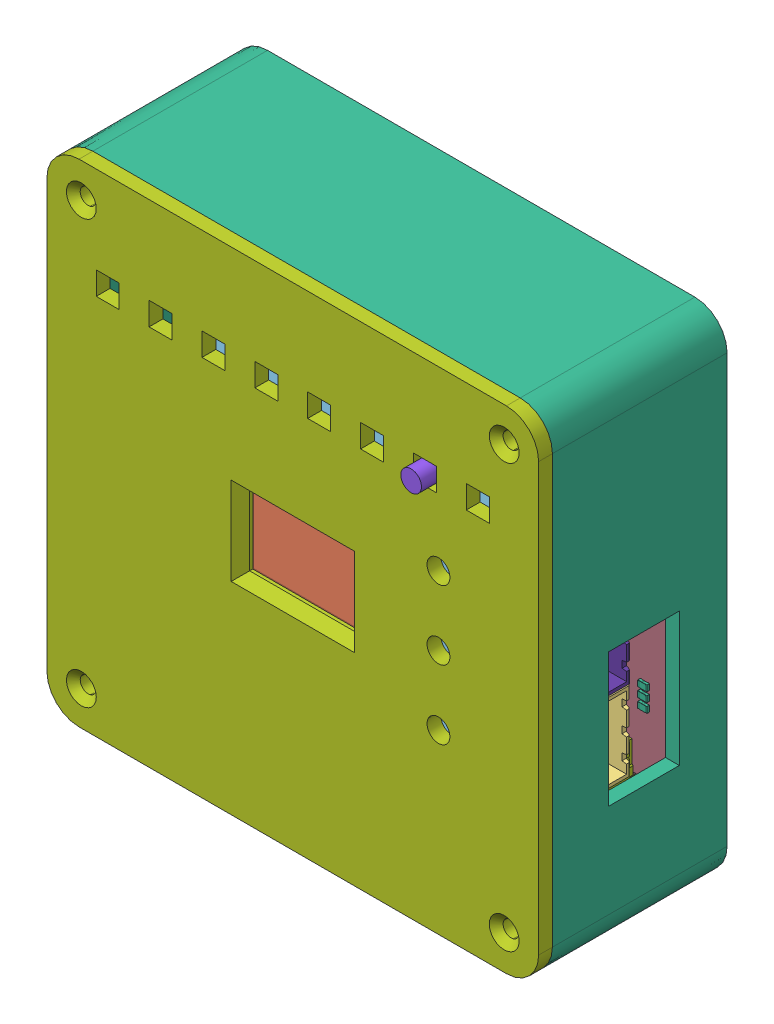
SolidWorks assembly SCATOLA, configuration Default. Lengths in mm.
Overall size (106.97 106.97 60).
340 component instances, 47 part files, 13 mates.
Components (placement in the parent):
- 3D_SprinklerBoy_2025-06-05.step-1: 3D_SprinklerBoy_2025-06-05.step [Default] at (-81.1414 55.2441 94.0033) size (99.97 100.11 18.63)
  - C3~CAP-TH_BD5.0-P2.00-D0.8-FD~CAP-TH_BD5.0-P2.00-D0.5-FD-A~FMY4.step-1: C3~CAP-TH_BD5.0-P2.00-D0.8-FD~CAP-TH_BD5.0-P2.00-D0.5-FD-A~FMY4.step [Default] at (9.652 -64.1351 1.5862) x (-1 0 0) z (0 0 1) size (5.01 5.01 16.01)
    - CAP-TH_BD5.0-P2.00-D0.8-FD~CAP-TH_BD5.0-P2.00-D0.5-FD-A~FMY4.step-1: CAP-TH_BD5.0-P2.00-D0.8-FD~CAP-TH_BD5.0-P2.00-D0.5-FD-A~FMY4.step [Default] at origin size (5.01 5.01 16.01)
  - C3~CAP-TH_BD5.0-P2.00-D0.8-FD~CAP-TH_BD5.0-P2.00-D0.5-FD-A~FMY4.step-2: C3~CAP-TH_BD5.0-P2.00-D0.8-FD~CAP-TH_BD5.0-P2.00-D0.5-FD-A~FMY4.step [Default] at (21.082 -57.5311 1.5862) size (5.01 5.01 16.01)
    - CAP-TH_BD5.0-P2.00-D0.8-FD~CAP-TH_BD5.0-P2.00-D0.5-FD-A~FMY4.step-1: CAP-TH_BD5.0-P2.00-D0.8-FD~CAP-TH_BD5.0-P2.00-D0.5-FD-A~FMY4.step [Default] at origin size (5.01 5.01 16.01)
  - C3~CAP-TH_BD5.0-P2.00-D0.8-FD~CAP-TH_BD5.0-P2.00-D0.5-FD-A~FMY4.step-3: C3~CAP-TH_BD5.0-P2.00-D0.8-FD~CAP-TH_BD5.0-P2.00-D0.5-FD-A~FMY4.step [Default] at (29.9721 -54.3561 1.5862) x (-1 0 0) z (0 0 1) size (5.01 5.01 16.01)
    - CAP-TH_BD5.0-P2.00-D0.8-FD~CAP-TH_BD5.0-P2.00-D0.5-FD-A~FMY4.step-1: CAP-TH_BD5.0-P2.00-D0.8-FD~CAP-TH_BD5.0-P2.00-D0.5-FD-A~FMY4.step [Default] at origin size (5.01 5.01 16.01)
  - D6~SMA_L4.3-W2.5-LS5.0-RD~SMA_L4.3-W2.5-LS5.0-RD-1~FMY4.step-1: D6~SMA_L4.3-W2.5-LS5.0-RD~SMA_L4.3-W2.5-LS5.0-RD-1~FMY4.step [Default] at (7.493 -57.2771 1.5862) x (-1 0 0) z (0 0 1) size (5.2 2.5 2.1)
    - SMA_L4.3-W2.5-LS5.0-RD~SMA_L4.3-W2.5-LS5.0-RD-1~FMY4.step-1: SMA_L4.3-W2.5-LS5.0-RD~SMA_L4.3-W2.5-LS5.0-RD-1~FMY4.step [Default] at origin size (5.2 2.5 2.1)
  - F3~FUSE-TH_5X20RHOSFUSECLIP-SEAT~FUSE-TH_5X20~FMY4.step-1: F3~FUSE-TH_5X20RHOSFUSECLIP-SEAT~FUSE-TH_5X20~FMY4.step [Default] at (21.4549 -78.9722 1.5862) size (5.86 6.2 13.03)
    - FUSE-TH_5X20RHOSFUSECLIP-SEAT~FUSE-TH_5X20~FMY4.step-1: FUSE-TH_5X20RHOSFUSECLIP-SEAT~FUSE-TH_5X20~FMY4.step [Default] at origin size (5.86 6.2 13.03)
  - F3~FUSE-TH_5X20RHOSFUSECLIP-SEAT~FUSE-TH_5X20~FMY4.step-2: F3~FUSE-TH_5X20RHOSFUSECLIP-SEAT~FUSE-TH_5X20~FMY4.step [Default] at (5.4755 -78.9722 1.5862) x (-1 0 0) z (0 0 1) size (5.86 6.2 13.03)
    - FUSE-TH_5X20RHOSFUSECLIP-SEAT~FUSE-TH_5X20~FMY4.step-1: FUSE-TH_5X20RHOSFUSECLIP-SEAT~FUSE-TH_5X20~FMY4.step [Default] at origin size (5.86 6.2 13.03)
  - H1~HDR-TH_3P-P2.54-V-M-1~HDR-M-2.54_1x3~FMY4.step-1: H1~HDR-TH_3P-P2.54-V-M-1~HDR-M-2.54_1x3~FMY4.step [Default] at (22.225 -41.0211 1.5862) x (-1 0 0) z (0 0 1) size (7.62 2.54 11.5)
    - HDR-TH_3P-P2.54-V-M-1~HDR-M-2.54_1x3~FMY4.step-1: HDR-TH_3P-P2.54-V-M-1~HDR-M-2.54_1x3~FMY4.step [Default] at origin size (7.62 2.54 11.5)
  - L1~L0805~R0805_L2.0-W1.3-H0.6~FMY4.step-1: L1~L0805~R0805_L2.0-W1.3-H0.6~FMY4.step [Default] at (94.3612 -84.9632 1.5862) x (0 -1 0) z (0 0 1) size (2 1.3 0.61)
    - L0805~R0805_L2.0-W1.3-H0.6~FMY4.step-1: L0805~R0805_L2.0-W1.3-H0.6~FMY4.step [Default] at origin size (2 1.3 0.61)
  - R41~R0805~R0805_L2.0-W1.3-H0.6~FMY4.step-1: R41~R0805~R0805_L2.0-W1.3-H0.6~FMY4.step [Default] at (68.4531 -13.716 1.5862) x (0 -1 0) z (0 0 1) size (2 1.3 0.61)
    - R0805_NEW~R0805_L2.0-W1.3-H0.6~FMY4.step-1: R0805_NEW~R0805_L2.0-W1.3-H0.6~FMY4.step [Default] at origin size (2 1.3 0.61)
  - R41~R0805~R0805_L2.0-W1.3-H0.6~FMY4.step-2: R41~R0805~R0805_L2.0-W1.3-H0.6~FMY4.step [Default] at (66.2941 -13.716 1.5862) x (0 -1 0) z (0 0 1) size (2 1.3 0.61)
    - R0805_NEW~R0805_L2.0-W1.3-H0.6~FMY4.step-1: R0805_NEW~R0805_L2.0-W1.3-H0.6~FMY4.step [Default] at origin size (2 1.3 0.61)
  - R41~R0805~R0805_L2.0-W1.3-H0.6~FMY4.step-3: R41~R0805~R0805_L2.0-W1.3-H0.6~FMY4.step [Default] at (86.8682 -15.621 1.5862) x (0 -1 0) z (0 0 1) size (2 1.3 0.61)
    - R0805_NEW~R0805_L2.0-W1.3-H0.6~FMY4.step-1: R0805_NEW~R0805_L2.0-W1.3-H0.6~FMY4.step [Default] at origin size (2 1.3 0.61)
  - R41~R0805~R0805_L2.0-W1.3-H0.6~FMY4.step-4: R41~R0805~R0805_L2.0-W1.3-H0.6~FMY4.step [Default] at (89.4082 -15.621 1.5862) x (0 -1 0) z (0 0 1) size (2 1.3 0.61)
    - R0805_NEW~R0805_L2.0-W1.3-H0.6~FMY4.step-1: R0805_NEW~R0805_L2.0-W1.3-H0.6~FMY4.step [Default] at origin size (2 1.3 0.61)
  - R41~R0805~R0805_L2.0-W1.3-H0.6~FMY4.step-5: R41~R0805~R0805_L2.0-W1.3-H0.6~FMY4.step [Default] at (89.4082 -11.811 1.5862) x (0 1 0) z (0 0 1) size (2 1.3 0.61)
    - R0805_NEW~R0805_L2.0-W1.3-H0.6~FMY4.step-1: R0805_NEW~R0805_L2.0-W1.3-H0.6~FMY4.step [Default] at origin size (2 1.3 0.61)
  - R41~R0805~R0805_L2.0-W1.3-H0.6~FMY4.step-6: R41~R0805~R0805_L2.0-W1.3-H0.6~FMY4.step [Default] at (86.8682 -11.811 1.5862) x (0 1 0) z (0 0 1) size (2 1.3 0.61)
    - R0805_NEW~R0805_L2.0-W1.3-H0.6~FMY4.step-1: R0805_NEW~R0805_L2.0-W1.3-H0.6~FMY4.step [Default] at origin size (2 1.3 0.61)
  - R41~R0805~R0805_L2.0-W1.3-H0.6~FMY4.step-7: R41~R0805~R0805_L2.0-W1.3-H0.6~FMY4.step [Default] at (80.8992 -26.9241 1.5862) x (-1 0 0) z (0 0 1) size (2 1.3 0.61)
    - R0805_NEW~R0805_L2.0-W1.3-H0.6~FMY4.step-1: R0805_NEW~R0805_L2.0-W1.3-H0.6~FMY4.step [Default] at origin size (2 1.3 0.61)
  - R41~R0805~R0805_L2.0-W1.3-H0.6~FMY4.step-8: R41~R0805~R0805_L2.0-W1.3-H0.6~FMY4.step [Default] at (78.2322 -48.2601 1.5862) x (0 -1 0) z (0 0 1) size (2 1.3 0.61)
    - R0805_NEW~R0805_L2.0-W1.3-H0.6~FMY4.step-1: R0805_NEW~R0805_L2.0-W1.3-H0.6~FMY4.step [Default] at origin size (2 1.3 0.61)
  - R41~R0805~R0805_L2.0-W1.3-H0.6~FMY4.step-9: R41~R0805~R0805_L2.0-W1.3-H0.6~FMY4.step [Default] at (73.9141 -48.2601 1.5862) x (0 -1 0) z (0 0 1) size (2 1.3 0.61)
    - R0805_NEW~R0805_L2.0-W1.3-H0.6~FMY4.step-1: R0805_NEW~R0805_L2.0-W1.3-H0.6~FMY4.step [Default] at origin size (2 1.3 0.61)
  - R41~R0805~R0805_L2.0-W1.3-H0.6~FMY4.step-10: R41~R0805~R0805_L2.0-W1.3-H0.6~FMY4.step [Default] at (93.2182 -67.3101 1.5862) size (2 1.3 0.61)
    - R0805_NEW~R0805_L2.0-W1.3-H0.6~FMY4.step-1: R0805_NEW~R0805_L2.0-W1.3-H0.6~FMY4.step [Default] at origin size (2 1.3 0.61)
  - R41~R0805~R0805_L2.0-W1.3-H0.6~FMY4.step-11: R41~R0805~R0805_L2.0-W1.3-H0.6~FMY4.step [Default] at (73.9141 -61.4681 1.5862) x (-1 0 0) z (0 0 1) size (2 1.3 0.61)
    - R0805_NEW~R0805_L2.0-W1.3-H0.6~FMY4.step-1: R0805_NEW~R0805_L2.0-W1.3-H0.6~FMY4.step [Default] at origin size (2 1.3 0.61)
  - R41~R0805~R0805_L2.0-W1.3-H0.6~FMY4.step-12: R41~R0805~R0805_L2.0-W1.3-H0.6~FMY4.step [Default] at (77.4702 -70.3581 1.5862) x (0 1 0) z (0 0 1) size (2 1.3 0.61)
    - R0805_NEW~R0805_L2.0-W1.3-H0.6~FMY4.step-1: R0805_NEW~R0805_L2.0-W1.3-H0.6~FMY4.step [Default] at origin size (2 1.3 0.61)
  - R41~R0805~R0805_L2.0-W1.3-H0.6~FMY4.step-13: R41~R0805~R0805_L2.0-W1.3-H0.6~FMY4.step [Default] at (80.2642 -72.0091 1.5862) x (0 -1 0) z (0 0 1) size (2 1.3 0.61)
    - R0805_NEW~R0805_L2.0-W1.3-H0.6~FMY4.step-1: R0805_NEW~R0805_L2.0-W1.3-H0.6~FMY4.step [Default] at origin size (2 1.3 0.61)
  - R41~R0805~R0805_L2.0-W1.3-H0.6~FMY4.step-14: R41~R0805~R0805_L2.0-W1.3-H0.6~FMY4.step [Default] at (82.4232 -72.0091 1.5862) x (0 -1 0) z (0 0 1) size (2 1.3 0.61)
    - R0805_NEW~R0805_L2.0-W1.3-H0.6~FMY4.step-1: R0805_NEW~R0805_L2.0-W1.3-H0.6~FMY4.step [Default] at origin size (2 1.3 0.61)
  - R41~R0805~R0805_L2.0-W1.3-H0.6~FMY4.step-15: R41~R0805~R0805_L2.0-W1.3-H0.6~FMY4.step [Default] at (85.3442 -70.3581 1.5862) x (0 1 0) z (0 0 1) size (2 1.3 0.61)
    - R0805_NEW~R0805_L2.0-W1.3-H0.6~FMY4.step-1: R0805_NEW~R0805_L2.0-W1.3-H0.6~FMY4.step [Default] at origin size (2 1.3 0.61)
  - R41~R0805~R0805_L2.0-W1.3-H0.6~FMY4.step-16: R41~R0805~R0805_L2.0-W1.3-H0.6~FMY4.step [Default] at (93.2182 -69.3421 1.5862) size (2 1.3 0.61)
    - R0805_NEW~R0805_L2.0-W1.3-H0.6~FMY4.step-1: R0805_NEW~R0805_L2.0-W1.3-H0.6~FMY4.step [Default] at origin size (2 1.3 0.61)
  - R41~R0805~R0805_L2.0-W1.3-H0.6~FMY4.step-17: R41~R0805~R0805_L2.0-W1.3-H0.6~FMY4.step [Default] at (93.2182 -71.3741 1.5862) size (2 1.3 0.61)
    - R0805_NEW~R0805_L2.0-W1.3-H0.6~FMY4.step-1: R0805_NEW~R0805_L2.0-W1.3-H0.6~FMY4.step [Default] at origin size (2 1.3 0.61)
  - R41~R0805~R0805_L2.0-W1.3-H0.6~FMY4.step-18: R41~R0805~R0805_L2.0-W1.3-H0.6~FMY4.step [Default] at (30.8611 -67.8181 1.5862) x (-1 0 0) z (0 0 1) size (2 1.3 0.61)
    - R0805_NEW~R0805_L2.0-W1.3-H0.6~FMY4.step-1: R0805_NEW~R0805_L2.0-W1.3-H0.6~FMY4.step [Default] at origin size (2 1.3 0.61)
  - R41~R0805~R0805_L2.0-W1.3-H0.6~FMY4.step-19: R41~R0805~R0805_L2.0-W1.3-H0.6~FMY4.step [Default] at (36.0681 -67.8181 1.5862) x (-1 0 0) z (0 0 1) size (2 1.3 0.61)
    - R0805_NEW~R0805_L2.0-W1.3-H0.6~FMY4.step-1: R0805_NEW~R0805_L2.0-W1.3-H0.6~FMY4.step [Default] at origin size (2 1.3 0.61)
  - R41~R0805~R0805_L2.0-W1.3-H0.6~FMY4.step-20: R41~R0805~R0805_L2.0-W1.3-H0.6~FMY4.step [Default] at (41.2751 -67.8181 1.5862) x (-1 0 0) z (0 0 1) size (2 1.3 0.61)
    - R0805_NEW~R0805_L2.0-W1.3-H0.6~FMY4.step-1: R0805_NEW~R0805_L2.0-W1.3-H0.6~FMY4.step [Default] at origin size (2 1.3 0.61)
  - R41~R0805~R0805_L2.0-W1.3-H0.6~FMY4.step-21: R41~R0805~R0805_L2.0-W1.3-H0.6~FMY4.step [Default] at (46.3551 -67.8181 1.5862) x (-1 0 0) z (0 0 1) size (2 1.3 0.61)
    - R0805_NEW~R0805_L2.0-W1.3-H0.6~FMY4.step-1: R0805_NEW~R0805_L2.0-W1.3-H0.6~FMY4.step [Default] at origin size (2 1.3 0.61)
  - R41~R0805~R0805_L2.0-W1.3-H0.6~FMY4.step-22: R41~R0805~R0805_L2.0-W1.3-H0.6~FMY4.step [Default] at (51.4351 -67.8181 1.5862) x (-1 0 0) z (0 0 1) size (2 1.3 0.61)
    - R0805_NEW~R0805_L2.0-W1.3-H0.6~FMY4.step-1: R0805_NEW~R0805_L2.0-W1.3-H0.6~FMY4.step [Default] at origin size (2 1.3 0.61)
  - R41~R0805~R0805_L2.0-W1.3-H0.6~FMY4.step-23: R41~R0805~R0805_L2.0-W1.3-H0.6~FMY4.step [Default] at (56.5151 -67.8181 1.5862) x (-1 0 0) z (0 0 1) size (2 1.3 0.61)
    - R0805_NEW~R0805_L2.0-W1.3-H0.6~FMY4.step-1: R0805_NEW~R0805_L2.0-W1.3-H0.6~FMY4.step [Default] at origin size (2 1.3 0.61)
  - R41~R0805~R0805_L2.0-W1.3-H0.6~FMY4.step-24: R41~R0805~R0805_L2.0-W1.3-H0.6~FMY4.step [Default] at (31.7501 -64.7701 1.5862) x (0 -1 0) z (0 0 1) size (2 1.3 0.61)
    - R0805_NEW~R0805_L2.0-W1.3-H0.6~FMY4.step-1: R0805_NEW~R0805_L2.0-W1.3-H0.6~FMY4.step [Default] at origin size (2 1.3 0.61)
  - R41~R0805~R0805_L2.0-W1.3-H0.6~FMY4.step-25: R41~R0805~R0805_L2.0-W1.3-H0.6~FMY4.step [Default] at (36.9571 -64.7701 1.5862) x (0 -1 0) z (0 0 1) size (2 1.3 0.61)
    - R0805_NEW~R0805_L2.0-W1.3-H0.6~FMY4.step-1: R0805_NEW~R0805_L2.0-W1.3-H0.6~FMY4.step [Default] at origin size (2 1.3 0.61)
  - R41~R0805~R0805_L2.0-W1.3-H0.6~FMY4.step-26: R41~R0805~R0805_L2.0-W1.3-H0.6~FMY4.step [Default] at (42.1641 -64.7701 1.5862) x (0 -1 0) z (0 0 1) size (2 1.3 0.61)
    - R0805_NEW~R0805_L2.0-W1.3-H0.6~FMY4.step-1: R0805_NEW~R0805_L2.0-W1.3-H0.6~FMY4.step [Default] at origin size (2 1.3 0.61)
  - R41~R0805~R0805_L2.0-W1.3-H0.6~FMY4.step-27: R41~R0805~R0805_L2.0-W1.3-H0.6~FMY4.step [Default] at (47.2441 -64.7701 1.5862) x (0 -1 0) z (0 0 1) size (2 1.3 0.61)
    - R0805_NEW~R0805_L2.0-W1.3-H0.6~FMY4.step-1: R0805_NEW~R0805_L2.0-W1.3-H0.6~FMY4.step [Default] at origin size (2 1.3 0.61)
  - R41~R0805~R0805_L2.0-W1.3-H0.6~FMY4.step-28: R41~R0805~R0805_L2.0-W1.3-H0.6~FMY4.step [Default] at (87.8842 -69.7231 1.5862) x (0 -1 0) z (0 0 1) size (2 1.3 0.61)
    - R0805_NEW~R0805_L2.0-W1.3-H0.6~FMY4.step-1: R0805_NEW~R0805_L2.0-W1.3-H0.6~FMY4.step [Default] at origin size (2 1.3 0.61)
  - R41~R0805~R0805_L2.0-W1.3-H0.6~FMY4.step-29: R41~R0805~R0805_L2.0-W1.3-H0.6~FMY4.step [Default] at (82.2962 -12.192 1.5862) x (-1 0 0) z (0 0 1) size (2 1.3 0.61)
    - R0805_NEW~R0805_L2.0-W1.3-H0.6~FMY4.step-1: R0805_NEW~R0805_L2.0-W1.3-H0.6~FMY4.step [Default] at origin size (2 1.3 0.61)
  - R41~R0805~R0805_L2.0-W1.3-H0.6~FMY4.step-30: R41~R0805~R0805_L2.0-W1.3-H0.6~FMY4.step [Default] at (82.2962 -10.033 1.5862) size (2 1.3 0.61)
    - R0805_NEW~R0805_L2.0-W1.3-H0.6~FMY4.step-1: R0805_NEW~R0805_L2.0-W1.3-H0.6~FMY4.step [Default] at origin size (2 1.3 0.61)
  - R41~R0805~R0805_L2.0-W1.3-H0.6~FMY4.step-31: R41~R0805~R0805_L2.0-W1.3-H0.6~FMY4.step [Default] at (61.7221 -67.8181 1.5862) x (-1 0 0) z (0 0 1) size (2 1.3 0.61)
    - R0805_NEW~R0805_L2.0-W1.3-H0.6~FMY4.step-1: R0805_NEW~R0805_L2.0-W1.3-H0.6~FMY4.step [Default] at origin size (2 1.3 0.61)
  - R41~R0805~R0805_L2.0-W1.3-H0.6~FMY4.step-32: R41~R0805~R0805_L2.0-W1.3-H0.6~FMY4.step [Default] at (66.9291 -67.8181 1.5862) x (-1 0 0) z (0 0 1) size (2 1.3 0.61)
    - R0805_NEW~R0805_L2.0-W1.3-H0.6~FMY4.step-1: R0805_NEW~R0805_L2.0-W1.3-H0.6~FMY4.step [Default] at origin size (2 1.3 0.61)
  - R41~R0805~R0805_L2.0-W1.3-H0.6~FMY4.step-33: R41~R0805~R0805_L2.0-W1.3-H0.6~FMY4.step [Default] at (52.3241 -64.7701 1.5862) x (0 -1 0) z (0 0 1) size (2 1.3 0.61)
    - R0805_NEW~R0805_L2.0-W1.3-H0.6~FMY4.step-1: R0805_NEW~R0805_L2.0-W1.3-H0.6~FMY4.step [Default] at origin size (2 1.3 0.61)
  - R41~R0805~R0805_L2.0-W1.3-H0.6~FMY4.step-34: R41~R0805~R0805_L2.0-W1.3-H0.6~FMY4.step [Default] at (57.4041 -64.7701 1.5862) x (0 -1 0) z (0 0 1) size (2 1.3 0.61)
    - R0805_NEW~R0805_L2.0-W1.3-H0.6~FMY4.step-1: R0805_NEW~R0805_L2.0-W1.3-H0.6~FMY4.step [Default] at origin size (2 1.3 0.61)
  - R41~R0805~R0805_L2.0-W1.3-H0.6~FMY4.step-35: R41~R0805~R0805_L2.0-W1.3-H0.6~FMY4.step [Default] at (62.6111 -64.7701 1.5862) x (0 -1 0) z (0 0 1) size (2 1.3 0.61)
    - R0805_NEW~R0805_L2.0-W1.3-H0.6~FMY4.step-1: R0805_NEW~R0805_L2.0-W1.3-H0.6~FMY4.step [Default] at origin size (2 1.3 0.61)
  - R41~R0805~R0805_L2.0-W1.3-H0.6~FMY4.step-36: R41~R0805~R0805_L2.0-W1.3-H0.6~FMY4.step [Default] at (67.6911 -64.7701 1.5862) x (0 -1 0) z (0 0 1) size (2 1.3 0.61)
    - R0805_NEW~R0805_L2.0-W1.3-H0.6~FMY4.step-1: R0805_NEW~R0805_L2.0-W1.3-H0.6~FMY4.step [Default] at origin size (2 1.3 0.61)
  - R41~R0805~R0805_L2.0-W1.3-H0.6~FMY4.step-37: R41~R0805~R0805_L2.0-W1.3-H0.6~FMY4.step [Default] at (8.255 -28.4481 1.5862) x (-1 0 0) z (0 0 1) size (2 1.3 0.61)
    - R0805_NEW~R0805_L2.0-W1.3-H0.6~FMY4.step-1: R0805_NEW~R0805_L2.0-W1.3-H0.6~FMY4.step [Default] at origin size (2 1.3 0.61)
  - R41~R0805~R0805_L2.0-W1.3-H0.6~FMY4.step-38: R41~R0805~R0805_L2.0-W1.3-H0.6~FMY4.step [Default] at (13.589 -28.4481 1.5862) x (-1 0 0) z (0 0 1) size (2 1.3 0.61)
    - R0805_NEW~R0805_L2.0-W1.3-H0.6~FMY4.step-1: R0805_NEW~R0805_L2.0-W1.3-H0.6~FMY4.step [Default] at origin size (2 1.3 0.61)
  - R41~R0805~R0805_L2.0-W1.3-H0.6~FMY4.step-39: R41~R0805~R0805_L2.0-W1.3-H0.6~FMY4.step [Default] at (19.177 -28.4481 1.5862) x (-1 0 0) z (0 0 1) size (2 1.3 0.61)
    - R0805_NEW~R0805_L2.0-W1.3-H0.6~FMY4.step-1: R0805_NEW~R0805_L2.0-W1.3-H0.6~FMY4.step [Default] at origin size (2 1.3 0.61)
  - R41~R0805~R0805_L2.0-W1.3-H0.6~FMY4.step-40: R41~R0805~R0805_L2.0-W1.3-H0.6~FMY4.step [Default] at (24.638 -28.5751 1.5862) x (-1 0 0) z (0 0 1) size (2 1.3 0.61)
    - R0805_NEW~R0805_L2.0-W1.3-H0.6~FMY4.step-1: R0805_NEW~R0805_L2.0-W1.3-H0.6~FMY4.step [Default] at origin size (2 1.3 0.61)
  - R41~R0805~R0805_L2.0-W1.3-H0.6~FMY4.step-41: R41~R0805~R0805_L2.0-W1.3-H0.6~FMY4.step [Default] at (29.9721 -28.5751 1.5862) x (-1 0 0) z (0 0 1) size (2 1.3 0.61)
    - R0805_NEW~R0805_L2.0-W1.3-H0.6~FMY4.step-1: R0805_NEW~R0805_L2.0-W1.3-H0.6~FMY4.step [Default] at origin size (2 1.3 0.61)
  - R41~R0805~R0805_L2.0-W1.3-H0.6~FMY4.step-42: R41~R0805~R0805_L2.0-W1.3-H0.6~FMY4.step [Default] at (35.6871 -28.5751 1.5862) x (-1 0 0) z (0 0 1) size (2 1.3 0.61)
    - R0805_NEW~R0805_L2.0-W1.3-H0.6~FMY4.step-1: R0805_NEW~R0805_L2.0-W1.3-H0.6~FMY4.step [Default] at origin size (2 1.3 0.61)
  - R41~R0805~R0805_L2.0-W1.3-H0.6~FMY4.step-43: R41~R0805~R0805_L2.0-W1.3-H0.6~FMY4.step [Default] at (11.811 -12.065 1.5862) x (0 -1 0) z (0 0 1) size (2 1.3 0.61)
    - R0805_NEW~R0805_L2.0-W1.3-H0.6~FMY4.step-1: R0805_NEW~R0805_L2.0-W1.3-H0.6~FMY4.step [Default] at origin size (2 1.3 0.61)
  - R41~R0805~R0805_L2.0-W1.3-H0.6~FMY4.step-44: R41~R0805~R0805_L2.0-W1.3-H0.6~FMY4.step [Default] at (17.272 -11.938 1.5862) x (0 -1 0) z (0 0 1) size (2 1.3 0.61)
    - R0805_NEW~R0805_L2.0-W1.3-H0.6~FMY4.step-1: R0805_NEW~R0805_L2.0-W1.3-H0.6~FMY4.step [Default] at origin size (2 1.3 0.61)
  - R41~R0805~R0805_L2.0-W1.3-H0.6~FMY4.step-45: R41~R0805~R0805_L2.0-W1.3-H0.6~FMY4.step [Default] at (22.733 -11.938 1.5862) x (0 -1 0) z (0 0 1) size (2 1.3 0.61)
    - R0805_NEW~R0805_L2.0-W1.3-H0.6~FMY4.step-1: R0805_NEW~R0805_L2.0-W1.3-H0.6~FMY4.step [Default] at origin size (2 1.3 0.61)
  - R41~R0805~R0805_L2.0-W1.3-H0.6~FMY4.step-46: R41~R0805~R0805_L2.0-W1.3-H0.6~FMY4.step [Default] at (28.1941 -12.065 1.5862) x (0 -1 0) z (0 0 1) size (2 1.3 0.61)
    - R0805_NEW~R0805_L2.0-W1.3-H0.6~FMY4.step-1: R0805_NEW~R0805_L2.0-W1.3-H0.6~FMY4.step [Default] at origin size (2 1.3 0.61)
  - R41~R0805~R0805_L2.0-W1.3-H0.6~FMY4.step-47: R41~R0805~R0805_L2.0-W1.3-H0.6~FMY4.step [Default] at (33.6551 -12.065 1.5862) x (0 -1 0) z (0 0 1) size (2 1.3 0.61)
    - R0805_NEW~R0805_L2.0-W1.3-H0.6~FMY4.step-1: R0805_NEW~R0805_L2.0-W1.3-H0.6~FMY4.step [Default] at origin size (2 1.3 0.61)
  - R41~R0805~R0805_L2.0-W1.3-H0.6~FMY4.step-48: R41~R0805~R0805_L2.0-W1.3-H0.6~FMY4.step [Default] at (39.1161 -12.065 1.5862) x (0 -1 0) z (0 0 1) size (2 1.3 0.61)
    - R0805_NEW~R0805_L2.0-W1.3-H0.6~FMY4.step-1: R0805_NEW~R0805_L2.0-W1.3-H0.6~FMY4.step [Default] at origin size (2 1.3 0.61)
  - R41~R0805~R0805_L2.0-W1.3-H0.6~FMY4.step-49: R41~R0805~R0805_L2.0-W1.3-H0.6~FMY4.step [Default] at (41.0211 -28.5751 1.5862) x (-1 0 0) z (0 0 1) size (2 1.3 0.61)
    - R0805_NEW~R0805_L2.0-W1.3-H0.6~FMY4.step-1: R0805_NEW~R0805_L2.0-W1.3-H0.6~FMY4.step [Default] at origin size (2 1.3 0.61)
  - R41~R0805~R0805_L2.0-W1.3-H0.6~FMY4.step-50: R41~R0805~R0805_L2.0-W1.3-H0.6~FMY4.step [Default] at (44.7041 -12.065 1.5862) x (0 -1 0) z (0 0 1) size (2 1.3 0.61)
    - R0805_NEW~R0805_L2.0-W1.3-H0.6~FMY4.step-1: R0805_NEW~R0805_L2.0-W1.3-H0.6~FMY4.step [Default] at origin size (2 1.3 0.61)
  - R41~R0805~R0805_L2.0-W1.3-H0.6~FMY4.step-51: R41~R0805~R0805_L2.0-W1.3-H0.6~FMY4.step [Default] at (46.4821 -28.5751 1.5862) x (-1 0 0) z (0 0 1) size (2 1.3 0.61)
    - R0805_NEW~R0805_L2.0-W1.3-H0.6~FMY4.step-1: R0805_NEW~R0805_L2.0-W1.3-H0.6~FMY4.step [Default] at origin size (2 1.3 0.61)
  - R41~R0805~R0805_L2.0-W1.3-H0.6~FMY4.step-52: R41~R0805~R0805_L2.0-W1.3-H0.6~FMY4.step [Default] at (50.0381 -12.065 1.5862) x (0 -1 0) z (0 0 1) size (2 1.3 0.61)
    - R0805_NEW~R0805_L2.0-W1.3-H0.6~FMY4.step-1: R0805_NEW~R0805_L2.0-W1.3-H0.6~FMY4.step [Default] at origin size (2 1.3 0.61)
  - R41~R0805~R0805_L2.0-W1.3-H0.6~FMY4.step-53: R41~R0805~R0805_L2.0-W1.3-H0.6~FMY4.step [Default] at (14.605 -64.7701 1.5862) x (0 1 0) z (0 0 1) size (2 1.3 0.61)
    - R0805_NEW~R0805_L2.0-W1.3-H0.6~FMY4.step-1: R0805_NEW~R0805_L2.0-W1.3-H0.6~FMY4.step [Default] at origin size (2 1.3 0.61)
  - R41~R0805~R0805_L2.0-W1.3-H0.6~FMY4.step-54: R41~R0805~R0805_L2.0-W1.3-H0.6~FMY4.step [Default] at (72.1361 -11.811 1.5862) x (-1 0 0) z (0 0 1) size (2 1.3 0.61)
    - R0805_NEW~R0805_L2.0-W1.3-H0.6~FMY4.step-1: R0805_NEW~R0805_L2.0-W1.3-H0.6~FMY4.step [Default] at origin size (2 1.3 0.61)
  - R41~R0805~R0805_L2.0-W1.3-H0.6~FMY4.step-55: R41~R0805~R0805_L2.0-W1.3-H0.6~FMY4.step [Default] at (62.3571 -11.811 1.5862) size (2 1.3 0.61)
    - R0805_NEW~R0805_L2.0-W1.3-H0.6~FMY4.step-1: R0805_NEW~R0805_L2.0-W1.3-H0.6~FMY4.step [Default] at origin size (2 1.3 0.61)
  - R41~R0805~R0805_L2.0-W1.3-H0.6~FMY4.step-56: R41~R0805~R0805_L2.0-W1.3-H0.6~FMY4.step [Default] at (76.8352 -13.843 1.5862) x (0 1 0) z (0 0 1) size (2 1.3 0.61)
    - R0805_NEW~R0805_L2.0-W1.3-H0.6~FMY4.step-1: R0805_NEW~R0805_L2.0-W1.3-H0.6~FMY4.step [Default] at origin size (2 1.3 0.61)
  - L1~L0805~R0805_L2.0-W1.3-H0.6~FMY4.step-2: L1~L0805~R0805_L2.0-W1.3-H0.6~FMY4.step [Default] at (76.9622 -54.6101 1.5862) size (2 1.3 0.61)
    - L0805~R0805_L2.0-W1.3-H0.6~FMY4.step-1: L0805~R0805_L2.0-W1.3-H0.6~FMY4.step [Default] at origin size (2 1.3 0.61)
  - J1~RJ45-TH_HR911105A~RJ45-TH_HR911105A~FMY4.step-1: J1~RJ45-TH_HR911105A~RJ45-TH_HR911105A~FMY4.step [Default] at (83.2172 -87.0495 1.5862) size (15.86 21.59 17.14)
    - RJ45-TH_HR911105A~RJ45-TH_HR911105A~FMY4.step-1: RJ45-TH_HR911105A~RJ45-TH_HR911105A~FMY4.step [Default] at origin size (15.86 21.59 17.14)
  - L3~IND-SMD_L12.3-W12.3_SMDRI127~SMD-PIND_L12.5-W12.5-H8.0~FMY4.step-1: L3~IND-SMD_L12.3-W12.3_SMDRI127~SMD-PIND_L12.5-W12.5-H8.0~FMY4.step [Default] at (10.922 -45.2121 1.5862) size (12.57 12.5 8)
    - IND-SMD_L12.3-W12.3_SMDRI127~SMD-PIND_L12.5-W12.5-H8.0~FMY4.step-1: IND-SMD_L12.3-W12.3_SMDRI127~SMD-PIND_L12.5-W12.5-H8.0~FMY4.step [Default] at origin size (12.57 12.5 8)
  - Q2~SOT-23-3_L2.9-W1.3-P1.90-LS2.4-BR~SOT-23-3P_L2.9-W1.3-H1.0-LS2.4-P0.95~FMY4.step-1: Q2~SOT-23-3_L2.9-W1.3-P1.90-LS2.4-BR~SOT-23-3P_L2.9-W1.3-H1.0-LS2.4-P0.95~FMY4.step [Default] at (84.0742 -15.494 1.5862) x (0 1 0) z (0 0 1) size (2.5 2.89 1.05)
    - SOT-23-3_L2.9-W1.3-P1.90-LS2.4-BR~SOT-23-3P_L2.9-W1.3-H1.0-LS2.4-P0.95~FMY4.step-1: SOT-23-3_L2.9-W1.3-P1.90-LS2.4-BR~SOT-23-3P_L2.9-W1.3-H1.0-LS2.4-P0.95~FMY4.step [Default] at origin size (2.5 2.89 1.05)
  - Q2~SOT-23-3_L2.9-W1.3-P1.90-LS2.4-BR~SOT-23-3P_L2.9-W1.3-H1.0-LS2.4-P0.95~FMY4.step-2: Q2~SOT-23-3_L2.9-W1.3-P1.90-LS2.4-BR~SOT-23-3P_L2.9-W1.3-H1.0-LS2.4-P0.95~FMY4.step [Default] at (80.6452 -15.494 1.5862) x (0 1 0) z (0 0 1) size (2.5 2.89 1.05)
    - SOT-23-3_L2.9-W1.3-P1.90-LS2.4-BR~SOT-23-3P_L2.9-W1.3-H1.0-LS2.4-P0.95~FMY4.step-1: SOT-23-3_L2.9-W1.3-P1.90-LS2.4-BR~SOT-23-3P_L2.9-W1.3-H1.0-LS2.4-P0.95~FMY4.step [Default] at origin size (2.5 2.89 1.05)
  - U3~WIFI-SMD_ESP32-WROOM-32UE~WIFI-SMD_L19.2-18.0-H3.2-ESP32-WROOM-32UE~FMY4.step-1: U3~WIFI-SMD_ESP32-WROOM-32UE~WIFI-SMD_L19.2-18.0-H3.2-ESP32-WROOM-32UE~FMY4.step [Default] at (89.6622 -38.1001 1.5862) x (0 -1 0) z (0 0 1) size (18 19.2 3.2)
    - WIFI-SMD_ESP32-WROOM-32UE~WIFI-SMD_L19.2-18.0-H3.2-ESP32-WROOM-32UE~FMY4.step-1: WIFI-SMD_ESP32-WROOM-32UE~WIFI-SMD_L19.2-18.0-H3.2-ESP32-WROOM-32UE~FMY4.step [Default] at origin size (18 19.2 3.2)
  - U4~QFN-24_L4.0-W4.0-P0.50-TL-EP2.5~VFQFN-24_L4.0-W4.0-P0.50-TL-EP2.1~FMY4.step-1: U4~QFN-24_L4.0-W4.0-P0.50-TL-EP2.5~VFQFN-24_L4.0-W4.0-P0.50-TL-EP2.1~FMY4.step [Default] at (80.9139 -61.6777 1.5862) x (-1 0 0) z (0 0 1) size (4.02 4.02 1.02)
    - QFN-24_L4.0-W4.0-P0.50-TL-EP2.5~VFQFN-24_L4.0-W4.0-P0.50-TL-EP2.1~FMY4.step-1: QFN-24_L4.0-W4.0-P0.50-TL-EP2.5~VFQFN-24_L4.0-W4.0-P0.50-TL-EP2.1~FMY4.step [Default] at origin size (4.02 4.02 1.02)
  - U13~SOP-4_L6.4-W4.6-P2.54-LS10.2-BL~SOP-4_L6.5-W4.6-H4.5-P2.54-LS10.2-TL~FMY4.step-1: U13~SOP-4_L6.4-W4.6-P2.54-LS10.2-BL~SOP-4_L6.5-W4.6-H4.5-P2.54-LS10.2-TL~FMY4.step [Default] at (26.9241 -20.32 1.5862) x (-1 0 0) z (0 0 1) size (4.6 10.3 4.64)
    - SOP-4_L6.4-W4.6-P2.54-LS10.2-BL~SOP-4_L6.5-W4.6-H4.5-P2.54-LS10.2-TL~FMY4.step-1: SOP-4_L6.4-W4.6-P2.54-LS10.2-BL~SOP-4_L6.5-W4.6-H4.5-P2.54-LS10.2-TL~FMY4.step [Default] at origin size (4.6 10.3 4.64)
  - U13~SOP-4_L6.4-W4.6-P2.54-LS10.2-BL~SOP-4_L6.5-W4.6-H4.5-P2.54-LS10.2-TL~FMY4.step-2: U13~SOP-4_L6.4-W4.6-P2.54-LS10.2-BL~SOP-4_L6.5-W4.6-H4.5-P2.54-LS10.2-TL~FMY4.step [Default] at (10.4734 -20.2632 1.5862) x (-1 0 0) z (0 0 1) size (4.6 10.3 4.64)
    - SOP-4_L6.4-W4.6-P2.54-LS10.2-BL~SOP-4_L6.5-W4.6-H4.5-P2.54-LS10.2-TL~FMY4.step-1: SOP-4_L6.4-W4.6-P2.54-LS10.2-BL~SOP-4_L6.5-W4.6-H4.5-P2.54-LS10.2-TL~FMY4.step [Default] at origin size (4.6 10.3 4.64)
  - U13~SOP-4_L6.4-W4.6-P2.54-LS10.2-BL~SOP-4_L6.5-W4.6-H4.5-P2.54-LS10.2-TL~FMY4.step-3: U13~SOP-4_L6.4-W4.6-P2.54-LS10.2-BL~SOP-4_L6.5-W4.6-H4.5-P2.54-LS10.2-TL~FMY4.step [Default] at (16.002 -20.32 1.5862) x (-1 0 0) z (0 0 1) size (4.6 10.3 4.64)
    - SOP-4_L6.4-W4.6-P2.54-LS10.2-BL~SOP-4_L6.5-W4.6-H4.5-P2.54-LS10.2-TL~FMY4.step-1: SOP-4_L6.4-W4.6-P2.54-LS10.2-BL~SOP-4_L6.5-W4.6-H4.5-P2.54-LS10.2-TL~FMY4.step [Default] at origin size (4.6 10.3 4.64)
  - U13~SOP-4_L6.4-W4.6-P2.54-LS10.2-BL~SOP-4_L6.5-W4.6-H4.5-P2.54-LS10.2-TL~FMY4.step-4: U13~SOP-4_L6.4-W4.6-P2.54-LS10.2-BL~SOP-4_L6.5-W4.6-H4.5-P2.54-LS10.2-TL~FMY4.step [Default] at (32.3851 -20.32 1.5862) x (-1 0 0) z (0 0 1) size (4.6 10.3 4.64)
    - SOP-4_L6.4-W4.6-P2.54-LS10.2-BL~SOP-4_L6.5-W4.6-H4.5-P2.54-LS10.2-TL~FMY4.step-1: SOP-4_L6.4-W4.6-P2.54-LS10.2-BL~SOP-4_L6.5-W4.6-H4.5-P2.54-LS10.2-TL~FMY4.step [Default] at origin size (4.6 10.3 4.64)
  - U13~SOP-4_L6.4-W4.6-P2.54-LS10.2-BL~SOP-4_L6.5-W4.6-H4.5-P2.54-LS10.2-TL~FMY4.step-5: U13~SOP-4_L6.4-W4.6-P2.54-LS10.2-BL~SOP-4_L6.5-W4.6-H4.5-P2.54-LS10.2-TL~FMY4.step [Default] at (37.8461 -20.32 1.5862) x (-1 0 0) z (0 0 1) size (4.6 10.3 4.64)
    - SOP-4_L6.4-W4.6-P2.54-LS10.2-BL~SOP-4_L6.5-W4.6-H4.5-P2.54-LS10.2-TL~FMY4.step-1: SOP-4_L6.4-W4.6-P2.54-LS10.2-BL~SOP-4_L6.5-W4.6-H4.5-P2.54-LS10.2-TL~FMY4.step [Default] at origin size (4.6 10.3 4.64)
  - U13~SOP-4_L6.4-W4.6-P2.54-LS10.2-BL~SOP-4_L6.5-W4.6-H4.5-P2.54-LS10.2-TL~FMY4.step-6: U13~SOP-4_L6.4-W4.6-P2.54-LS10.2-BL~SOP-4_L6.5-W4.6-H4.5-P2.54-LS10.2-TL~FMY4.step [Default] at (43.3071 -20.32 1.5862) x (-1 0 0) z (0 0 1) size (4.6 10.3 4.64)
    - SOP-4_L6.4-W4.6-P2.54-LS10.2-BL~SOP-4_L6.5-W4.6-H4.5-P2.54-LS10.2-TL~FMY4.step-1: SOP-4_L6.4-W4.6-P2.54-LS10.2-BL~SOP-4_L6.5-W4.6-H4.5-P2.54-LS10.2-TL~FMY4.step [Default] at origin size (4.6 10.3 4.64)
  - U13~SOP-4_L6.4-W4.6-P2.54-LS10.2-BL~SOP-4_L6.5-W4.6-H4.5-P2.54-LS10.2-TL~FMY4.step-7: U13~SOP-4_L6.4-W4.6-P2.54-LS10.2-BL~SOP-4_L6.5-W4.6-H4.5-P2.54-LS10.2-TL~FMY4.step [Default] at (48.7421 -20.3683 1.5862) x (-1 0 0) z (0 0 1) size (4.6 10.3 4.64)
    - SOP-4_L6.4-W4.6-P2.54-LS10.2-BL~SOP-4_L6.5-W4.6-H4.5-P2.54-LS10.2-TL~FMY4.step-1: SOP-4_L6.4-W4.6-P2.54-LS10.2-BL~SOP-4_L6.5-W4.6-H4.5-P2.54-LS10.2-TL~FMY4.step [Default] at origin size (4.6 10.3 4.64)
  - U13~SOP-4_L6.4-W4.6-P2.54-LS10.2-BL~SOP-4_L6.5-W4.6-H4.5-P2.54-LS10.2-TL~FMY4.step-8: U13~SOP-4_L6.4-W4.6-P2.54-LS10.2-BL~SOP-4_L6.5-W4.6-H4.5-P2.54-LS10.2-TL~FMY4.step [Default] at (21.463 -20.32 1.5862) x (-1 0 0) z (0 0 1) size (4.6 10.3 4.64)
    - SOP-4_L6.4-W4.6-P2.54-LS10.2-BL~SOP-4_L6.5-W4.6-H4.5-P2.54-LS10.2-TL~FMY4.step-1: SOP-4_L6.4-W4.6-P2.54-LS10.2-BL~SOP-4_L6.5-W4.6-H4.5-P2.54-LS10.2-TL~FMY4.step [Default] at origin size (4.6 10.3 4.64)
  - U2~SOT-223-4_L6.5-W3.5-P2.30-LS7.0-BR~SOT-223-4P_L6.5-W3.5-H1.6-LS7.0-P2.30~FMY4.step-1: U2~SOT-223-4_L6.5-W3.5-P2.30-LS7.0-BR~SOT-223-4P_L6.5-W3.5-H1.6-LS7.0-P2.30~FMY4.step [Default] at (35.8141 -50.2921 1.5862) x (0 1 0) z (0 0 1) size (7.11 6.5 1.75)
    - SOT-223-4_L6.5-W3.5-P2.30-LS7.0-BR~SOT-223-4P_L6.5-W3.5-H1.6-LS7.0-P2.30~FMY4.step-1: SOT-223-4_L6.5-W3.5-P2.30-LS7.0-BR~SOT-223-4P_L6.5-W3.5-H1.6-LS7.0-P2.30~FMY4.step [Default] at origin size (7.11 6.5 1.75)
  - U8~SMA_L4.5-W2.7-LS5.1-RD~SMA_L4.5-W2.7-LS5.1-RD~FMY4.step-1: U8~SMA_L4.5-W2.7-LS5.1-RD~SMA_L4.5-W2.7-LS5.1-RD~FMY4.step [Default] at (12.954 -72.3901 1.5862) size (5.1 2.7 2.2)
    - SMA_L4.5-W2.7-LS5.1-RD~SMA_L4.5-W2.7-LS5.1-RD~FMY4.step-1: SMA_L4.5-W2.7-LS5.1-RD~SMA_L4.5-W2.7-LS5.1-RD~FMY4.step [Default] at origin size (5.1 2.7 2.2)
  - U20~TSSOP-16_L5.0-W4.4-P0.65-LS6.4-BL~TSSOP-16_L5.0-W4.4-H1.0-LS6.4-P0.65~FMY4.step-1: U20~TSSOP-16_L5.0-W4.4-P0.65-LS6.4-BL~TSSOP-16_L5.0-W4.4-H1.0-LS6.4-P0.65~FMY4.step [Default] at (54.6101 -57.0231 1.5862) x (0 -1 0) z (0 0 1) size (0.76 0.76 0.76)
    - TSSOP-16_L5.0-W4.4-P0.65-LS6.4-BL~TSSOP-16_L5.0-W4.4-H1.0-LS6.4-P0.65~FMY4.step-1: TSSOP-16_L5.0-W4.4-P0.65-LS6.4-BL~TSSOP-16_L5.0-W4.4-H1.0-LS6.4-P0.65~FMY4.step [Default] at origin size (0.76 0.76 0.76)
  - U7~SOIC-8_L5.0-W4.0-P1.27-LS6.0-BL~SOIC-8_L4.9-W3.9-H1.7-LS6.0-P1.27~FMY4.step-1: U7~SOIC-8_L5.0-W4.0-P1.27-LS6.0-BL~SOIC-8_L4.9-W3.9-H1.7-LS6.0-P1.27~FMY4.step [Default] at (14.859 -57.0231 1.5862) size (4.81 6 1.72)
    - SOIC-8_L5.0-W4.0-P1.27-LS6.0-BL~SOIC-8_L4.9-W3.9-H1.7-LS6.0-P1.27~FMY4.step-1: SOIC-8_L5.0-W4.0-P1.27-LS6.0-BL~SOIC-8_L4.9-W3.9-H1.7-LS6.0-P1.27~FMY4.step [Default] at origin size (4.81 6 1.72)
  - U5~SOT-89-3_L4.5-W2.5-P1.50-LS4.2-BR~SOT-89-3_L4.3-W2.5-H1.6-LS4.1-P1.50~FMY4.step-1: U5~SOT-89-3_L4.5-W2.5-P1.50-LS4.2-BR~SOT-89-3_L4.3-W2.5-H1.6-LS4.1-P1.50~FMY4.step [Default] at (36.0681 -72.3901 1.5862) x (0 -1 0) z (0 0 1) size (4.1 4.3 1.61)
    - SOT-89-3_L4.5-W2.5-P1.50-LS4.2-BR~SOT-89-3_L4.3-W2.5-H1.6-LS4.1-P1.50~FMY4.step-1: SOT-89-3_L4.5-W2.5-P1.50-LS4.2-BR~SOT-89-3_L4.3-W2.5-H1.6-LS4.1-P1.50~FMY4.step [Default] at origin size (4.1 4.3 1.61)
  - U5~SOT-89-3_L4.5-W2.5-P1.50-LS4.2-BR~SOT-89-3_L4.3-W2.5-H1.6-LS4.1-P1.50~FMY4.step-2: U5~SOT-89-3_L4.5-W2.5-P1.50-LS4.2-BR~SOT-89-3_L4.3-W2.5-H1.6-LS4.1-P1.50~FMY4.step [Default] at (41.2751 -72.3901 1.5862) x (0 -1 0) z (0 0 1) size (4.1 4.3 1.61)
    - SOT-89-3_L4.5-W2.5-P1.50-LS4.2-BR~SOT-89-3_L4.3-W2.5-H1.6-LS4.1-P1.50~FMY4.step-1: SOT-89-3_L4.5-W2.5-P1.50-LS4.2-BR~SOT-89-3_L4.3-W2.5-H1.6-LS4.1-P1.50~FMY4.step [Default] at origin size (4.1 4.3 1.61)
  - U5~SOT-89-3_L4.5-W2.5-P1.50-LS4.2-BR~SOT-89-3_L4.3-W2.5-H1.6-LS4.1-P1.50~FMY4.step-3: U5~SOT-89-3_L4.5-W2.5-P1.50-LS4.2-BR~SOT-89-3_L4.3-W2.5-H1.6-LS4.1-P1.50~FMY4.step [Default] at (46.3551 -72.3901 1.5862) x (0 -1 0) z (0 0 1) size (4.1 4.3 1.61)
    - SOT-89-3_L4.5-W2.5-P1.50-LS4.2-BR~SOT-89-3_L4.3-W2.5-H1.6-LS4.1-P1.50~FMY4.step-1: SOT-89-3_L4.5-W2.5-P1.50-LS4.2-BR~SOT-89-3_L4.3-W2.5-H1.6-LS4.1-P1.50~FMY4.step [Default] at origin size (4.1 4.3 1.61)
  - U5~SOT-89-3_L4.5-W2.5-P1.50-LS4.2-BR~SOT-89-3_L4.3-W2.5-H1.6-LS4.1-P1.50~FMY4.step-4: U5~SOT-89-3_L4.5-W2.5-P1.50-LS4.2-BR~SOT-89-3_L4.3-W2.5-H1.6-LS4.1-P1.50~FMY4.step [Default] at (51.4351 -72.3901 1.5862) x (0 -1 0) z (0 0 1) size (4.1 4.3 1.61)
    - SOT-89-3_L4.5-W2.5-P1.50-LS4.2-BR~SOT-89-3_L4.3-W2.5-H1.6-LS4.1-P1.50~FMY4.step-1: SOT-89-3_L4.5-W2.5-P1.50-LS4.2-BR~SOT-89-3_L4.3-W2.5-H1.6-LS4.1-P1.50~FMY4.step [Default] at origin size (4.1 4.3 1.61)
  - U5~SOT-89-3_L4.5-W2.5-P1.50-LS4.2-BR~SOT-89-3_L4.3-W2.5-H1.6-LS4.1-P1.50~FMY4.step-5: U5~SOT-89-3_L4.5-W2.5-P1.50-LS4.2-BR~SOT-89-3_L4.3-W2.5-H1.6-LS4.1-P1.50~FMY4.step [Default] at (56.5151 -72.3901 1.5862) x (0 -1 0) z (0 0 1) size (4.1 4.3 1.61)
    - SOT-89-3_L4.5-W2.5-P1.50-LS4.2-BR~SOT-89-3_L4.3-W2.5-H1.6-LS4.1-P1.50~FMY4.step-1: SOT-89-3_L4.5-W2.5-P1.50-LS4.2-BR~SOT-89-3_L4.3-W2.5-H1.6-LS4.1-P1.50~FMY4.step [Default] at origin size (4.1 4.3 1.61)
  - U5~SOT-89-3_L4.5-W2.5-P1.50-LS4.2-BR~SOT-89-3_L4.3-W2.5-H1.6-LS4.1-P1.50~FMY4.step-6: U5~SOT-89-3_L4.5-W2.5-P1.50-LS4.2-BR~SOT-89-3_L4.3-W2.5-H1.6-LS4.1-P1.50~FMY4.step [Default] at (61.7221 -72.3901 1.5862) x (0 -1 0) z (0 0 1) size (4.1 4.3 1.61)
    - SOT-89-3_L4.5-W2.5-P1.50-LS4.2-BR~SOT-89-3_L4.3-W2.5-H1.6-LS4.1-P1.50~FMY4.step-1: SOT-89-3_L4.5-W2.5-P1.50-LS4.2-BR~SOT-89-3_L4.3-W2.5-H1.6-LS4.1-P1.50~FMY4.step [Default] at origin size (4.1 4.3 1.61)
  - U5~SOT-89-3_L4.5-W2.5-P1.50-LS4.2-BR~SOT-89-3_L4.3-W2.5-H1.6-LS4.1-P1.50~FMY4.step-7: U5~SOT-89-3_L4.5-W2.5-P1.50-LS4.2-BR~SOT-89-3_L4.3-W2.5-H1.6-LS4.1-P1.50~FMY4.step [Default] at (67.0561 -72.3901 1.5862) x (0 -1 0) z (0 0 1) size (4.1 4.3 1.61)
    - SOT-89-3_L4.5-W2.5-P1.50-LS4.2-BR~SOT-89-3_L4.3-W2.5-H1.6-LS4.1-P1.50~FMY4.step-1: SOT-89-3_L4.5-W2.5-P1.50-LS4.2-BR~SOT-89-3_L4.3-W2.5-H1.6-LS4.1-P1.50~FMY4.step [Default] at origin size (4.1 4.3 1.61)
  - U5~SOT-89-3_L4.5-W2.5-P1.50-LS4.2-BR~SOT-89-3_L4.3-W2.5-H1.6-LS4.1-P1.50~FMY4.step-8: U5~SOT-89-3_L4.5-W2.5-P1.50-LS4.2-BR~SOT-89-3_L4.3-W2.5-H1.6-LS4.1-P1.50~FMY4.step [Default] at (30.8611 -72.3901 1.5862) x (0 -1 0) z (0 0 1) size (4.1 4.3 1.61)
    - SOT-89-3_L4.5-W2.5-P1.50-LS4.2-BR~SOT-89-3_L4.3-W2.5-H1.6-LS4.1-P1.50~FMY4.step-1: SOT-89-3_L4.5-W2.5-P1.50-LS4.2-BR~SOT-89-3_L4.3-W2.5-H1.6-LS4.1-P1.50~FMY4.step [Default] at origin size (4.1 4.3 1.61)
  - LED1~LED0805-R-RD~LED0805-RD_RED_XL-2012SURC-FJ~FMY4.step-1: LED1~LED0805-R-RD~LED0805-RD_RED_XL-2012SURC-FJ~FMY4.step [Default] at (76.878 -9.4688 1.5862) x (0 1 0) z (0 0 1) size (2.1 1.15 0.81)
    - LED0805-R-RD~LED0805-RD_RED_XL-2012SURC-FJ~FMY4.step-1: LED0805-R-RD~LED0805-RD_RED_XL-2012SURC-FJ~FMY4.step [Default] at origin size (2.1 1.15 0.81)
  - C14~C0805~C0805_L2.0-W1.3-H1.3~FMY4.step-1: C14~C0805~C0805_L2.0-W1.3-H1.3~FMY4.step [Default] at (62.2301 -24.003 1.5862) x (0 -1 0) z (0 0 1) size (2 1.3 1.3)
    - C0805~C0805_L2.0-W1.3-H1.3~FMY4.step-1: C0805~C0805_L2.0-W1.3-H1.3~FMY4.step [Default] at origin size (2 1.3 1.3)
  - C14~C0805~C0805_L2.0-W1.3-H1.3~FMY4.step-2: C14~C0805~C0805_L2.0-W1.3-H1.3~FMY4.step [Default] at (96.0122 -25.4001 1.5862) x (-1 0 0) z (0 0 1) size (2 1.3 1.3)
    - C0805~C0805_L2.0-W1.3-H1.3~FMY4.step-1: C0805~C0805_L2.0-W1.3-H1.3~FMY4.step [Default] at origin size (2 1.3 1.3)
  - C14~C0805~C0805_L2.0-W1.3-H1.3~FMY4.step-3: C14~C0805~C0805_L2.0-W1.3-H1.3~FMY4.step [Default] at (96.0122 -23.368 1.5862) x (-1 0 0) z (0 0 1) size (2 1.3 1.3)
    - C0805~C0805_L2.0-W1.3-H1.3~FMY4.step-1: C0805~C0805_L2.0-W1.3-H1.3~FMY4.step [Default] at origin size (2 1.3 1.3)
  - C14~C0805~C0805_L2.0-W1.3-H1.3~FMY4.step-4: C14~C0805~C0805_L2.0-W1.3-H1.3~FMY4.step [Default] at (81.0262 -56.0071 1.5862) x (0 -1 0) z (0 0 1) size (2 1.3 1.3)
    - C0805~C0805_L2.0-W1.3-H1.3~FMY4.step-1: C0805~C0805_L2.0-W1.3-H1.3~FMY4.step [Default] at origin size (2 1.3 1.3)
  - C14~C0805~C0805_L2.0-W1.3-H1.3~FMY4.step-5: C14~C0805~C0805_L2.0-W1.3-H1.3~FMY4.step [Default] at (83.1852 -54.8641 1.5862) x (0 -1 0) z (0 0 1) size (2 1.3 1.3)
    - C0805~C0805_L2.0-W1.3-H1.3~FMY4.step-1: C0805~C0805_L2.0-W1.3-H1.3~FMY4.step [Default] at origin size (2 1.3 1.3)
  - C14~C0805~C0805_L2.0-W1.3-H1.3~FMY4.step-6: C14~C0805~C0805_L2.0-W1.3-H1.3~FMY4.step [Default] at (76.9622 -56.8961 1.5862) size (2 1.3 1.3)
    - C0805~C0805_L2.0-W1.3-H1.3~FMY4.step-1: C0805~C0805_L2.0-W1.3-H1.3~FMY4.step [Default] at origin size (2 1.3 1.3)
  - C14~C0805~C0805_L2.0-W1.3-H1.3~FMY4.step-7: C14~C0805~C0805_L2.0-W1.3-H1.3~FMY4.step [Default] at (86.4872 -64.5161 1.5862) x (-1 0 0) z (0 0 1) size (2 1.3 1.3)
    - C0805~C0805_L2.0-W1.3-H1.3~FMY4.step-1: C0805~C0805_L2.0-W1.3-H1.3~FMY4.step [Default] at origin size (2 1.3 1.3)
  - C14~C0805~C0805_L2.0-W1.3-H1.3~FMY4.step-8: C14~C0805~C0805_L2.0-W1.3-H1.3~FMY4.step [Default] at (85.2172 -54.8641 1.5862) x (0 -1 0) z (0 0 1) size (2 1.3 1.3)
    - C0805~C0805_L2.0-W1.3-H1.3~FMY4.step-1: C0805~C0805_L2.0-W1.3-H1.3~FMY4.step [Default] at origin size (2 1.3 1.3)
  - C14~C0805~C0805_L2.0-W1.3-H1.3~FMY4.step-9: C14~C0805~C0805_L2.0-W1.3-H1.3~FMY4.step [Default] at (73.9141 -59.4361 1.5862) size (2 1.3 1.3)
    - C0805~C0805_L2.0-W1.3-H1.3~FMY4.step-1: C0805~C0805_L2.0-W1.3-H1.3~FMY4.step [Default] at origin size (2 1.3 1.3)
